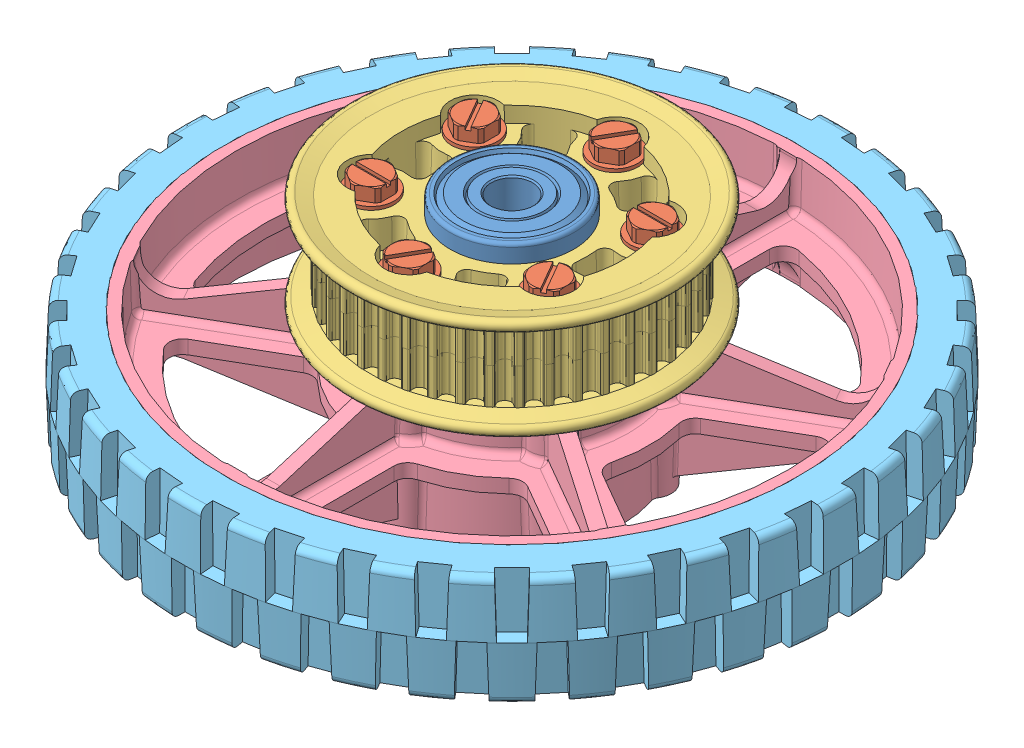
SolidWorks assembly 6 HiGrip and 42 HTD Pulley and Bearings-1, configuration Default. Lengths in mm.
Overall size (208.18 57.15 208.18).
13 component instances, 5 part files, 0 mates.
Components (placement in the parent):
- 1614Z Bearing-1-1: 1614Z Bearing-1 [Default] at (-8.55 -38.206 8.553) x (0.797444 0 -0.603394) z (0 1 0) size (28.57 28.57 9.53)
- 10-24 Hex Washer Rolling x 1-25_93882A213-1-1: 10-24 Hex Washer Rolling x 1-25_93882A213-1 [Default] at (12.0722 9.7619 -3.3533) x (1 0 0) z (0 1 0) size (10.52 10.52 35.59)
- 10-24 Hex Washer Rolling x 1-25_93882A213-1-2: 10-24 Hex Washer Rolling x 1-25_93882A213-1 [Default] at (-8.55 9.7619 -15.2595) x (0.5 0 -0.866025) z (0 1 0) size (10.52 10.52 35.59)
- 10-24 Hex Washer Rolling x 1-25_93882A213-1-3: 10-24 Hex Washer Rolling x 1-25_93882A213-1 [Default] at (12.0722 9.7619 20.4592) x (0.5 0 0.866025) z (0 1 0) size (10.52 10.52 35.59)
- 10-24 Hex Washer Rolling x 1-25_93882A213-1-4: 10-24 Hex Washer Rolling x 1-25_93882A213-1 [Default] at (-29.1722 9.7619 20.4592) x (-1 0 0) z (0 1 0) size (10.52 10.52 35.59)
- 42 tooth HTD Pulley half-1-1: 42 tooth HTD Pulley half-1 [Default] at (-8.55 10.7779 8.553) x (0 -1 0) z (0.5 0 0.866025) size (13 74.23 74.23)
- 10-24 Hex Washer Rolling x 1-25_93882A213-1-5: 10-24 Hex Washer Rolling x 1-25_93882A213-1 [Default] at (-8.55 9.7619 32.3655) x (-0.5 0 0.866025) z (0 1 0) size (10.52 10.52 35.59)
- 6 HiGrip Asm-1-1: 6 HiGrip Asm-1 [Default] at (9.3494 -30.192 1.7951) x (0.866025 0 -0.5) z (0 1 0) size (152.4 152.4 35.18)
  - 6in 2008 FIRST Hub-1-1: 6in 2008 FIRST Hub-1 [Default] at (-18.8802 3.0972 -4.839) size (139.7 139.7 35.18)
  - 6 HiGrip Tread-1-1: 6 HiGrip Tread-1 [Default] at (-18.8802 3.0972 -4.839) size (152.4 152.4 25.58)
- 1614Z Bearing-1-2: 1614Z Bearing-1 [Default] at (-8.55 9.1269 8.553) x (0.797444 0 -0.603394) z (0 1 0) size (28.57 28.57 9.53)
- 42 tooth HTD Pulley half-1-2: 42 tooth HTD Pulley half-1 [Default] at (-8.55 -5.8845 8.553) x (0 1 0) z (0.500073 0 0.865983) size (13 74.23 74.23)
- 10-24 Hex Washer Rolling x 1-25_93882A213-1-6: 10-24 Hex Washer Rolling x 1-25_93882A213-1 [Default] at (-29.1722 9.7619 -3.3533) x (-0.5 0 -0.866025) z (0 1 0) size (10.52 10.52 35.59)
